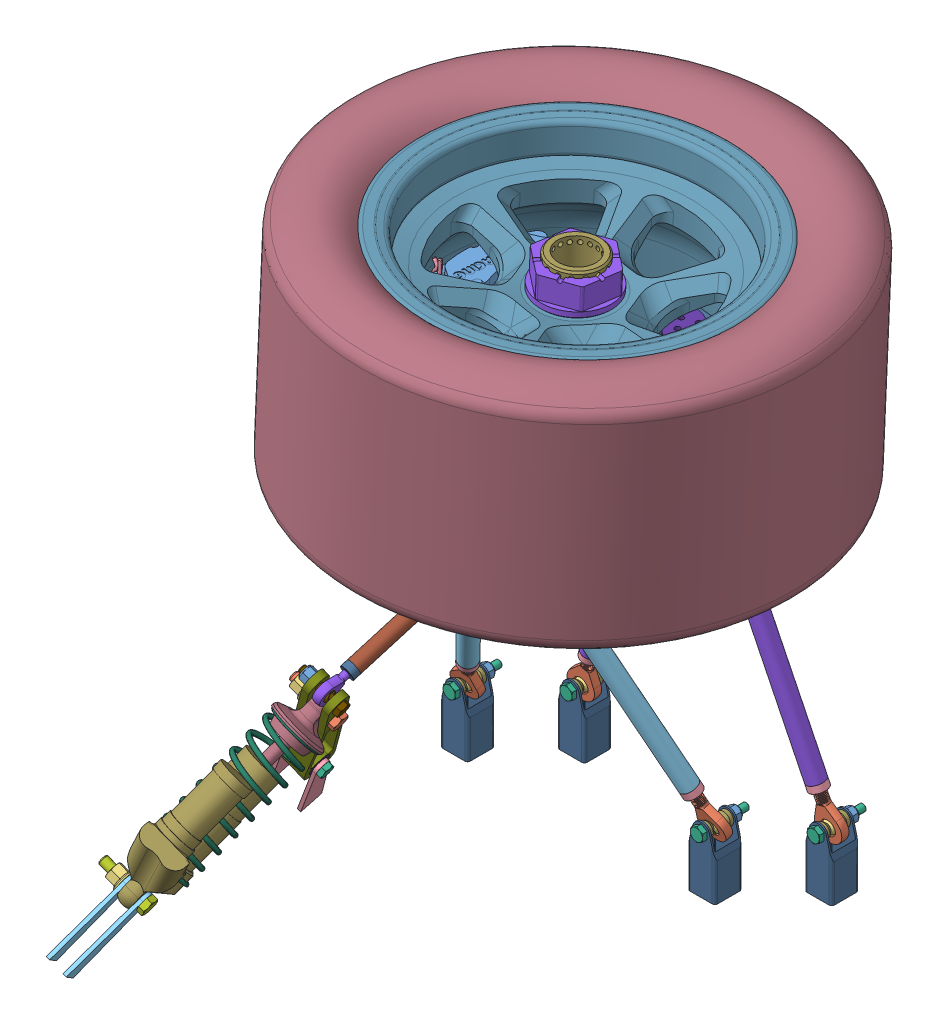
SolidWorks assembly WT-A0100-AC-Unsprung FRONT Axle Asszembly, configuration Default. Lengths in mm.
Overall size (1029.74 758.91 586.73).
149 component instances, 58 part files, 6 mates.
Components (placement in the parent):
- SP-A0200-AA-Front Axle Assembly-1: SP-A0200-AA-Front Axle Assembly [Default] at origin size (928.85 609.3 561.18)
  - Upper A-Arm^SP-A0200-AA-Front Axle Assembly-1: Upper A-Arm^SP-A0200-AA-Front Axle Assembly [Default] at (0 340.1778 -103.3743) x (1 0 0) z (0 -0.807933 0.589274) size (262.57 296.92 200.08) (virtual)
    - SP-Upper Apex Front-1: SP-Upper Apex Front [Default] at (789.6198 444.1063 49.8797) x (0.938572 -0.289882 0.187221) z (0 0.542537 0.840032) size (51.11 64.07 9.53)
    - MirrorFS-MALE ROD END UNF-3A, 0.3125x24-0.25D (XAM-4)1-1: MirrorFS-MALE ROD END UNF-3A, 0.3125x24-0.25D (XAM-4)1 [Default] at (903.9198 182.9597 218.5422) x (-0.938572 -0.289882 0.187221) z (0.345084 -0.78843 0.50921) size (26.22 11.39 62.85)
      - MirrorBody^MirrorFS-MALE ROD END UNF-3A, 0.3125x24-0.25D (XAM-4)1-1: MirrorBody^MirrorFS-MALE ROD END UNF-3A, 0.3125x24-0.25D (XAM-4)1 [Default] at origin size (26.22 9.76 62.85) (virtual)
      - MirrorBall^MirrorFS-MALE ROD END UNF-3A, 0.3125x24-0.25D (XAM-4)1-1: MirrorBall^MirrorFS-MALE ROD END UNF-3A, 0.3125x24-0.25D (XAM-4)1 [Default] x (0.874091 -0.054164 -0.482733) z (-0.485762 -0.097546 -0.868631) size (12.7 9.53 12.7) (virtual)
    - MirrorFS-MALE ROD END UNF-3A, 0.3125x24-0.25D (XAM-4)1-2: MirrorFS-MALE ROD END UNF-3A, 0.3125x24-0.25D (XAM-4)1 [Default] at (675.3198 182.9597 218.5422) x (0.938572 -0.289882 0.187221) z (-0.345084 -0.78843 0.50921) size (26.22 11.39 62.85)
      - MirrorBody^MirrorFS-MALE ROD END UNF-3A, 0.3125x24-0.25D (XAM-4)1-1: MirrorBody^MirrorFS-MALE ROD END UNF-3A, 0.3125x24-0.25D (XAM-4)1 [Default] at origin size (26.22 9.76 62.85) (virtual)
      - MirrorBall^MirrorFS-MALE ROD END UNF-3A, 0.3125x24-0.25D (XAM-4)1-1: MirrorBall^MirrorFS-MALE ROD END UNF-3A, 0.3125x24-0.25D (XAM-4)1 [Default] x (0.874091 -0.054164 -0.482733) z (-0.485762 -0.097546 -0.868631) size (12.7 9.53 12.7) (virtual)
    - SP-10003-AD-Threaded Insert-1: SP-10003-AD-Threaded Insert [A-Arm] at (690.6588 218.0055 195.9078) x (-0.938572 0.289882 -0.187221) z (-0.345084 -0.78843 0.50921) size (15.88 15.88 15.88)
    - SP-10003-AD-Threaded Insert-2: SP-10003-AD-Threaded Insert [A-Arm] at (888.5808 218.0055 195.9078) x (0 0.542537 0.840032) z (0.345084 -0.78843 0.50921) size (15.88 15.88 15.88)
    - SP-Upper A-Arm Tube-1: SP-Upper A-Arm Tube [Default] at (732.4698 313.533 134.2109) x (0 -0.542537 -0.840032) z (0.938572 -0.289882 0.187221) size (15.88 272.31 15.88)
    - SP-Upper A-Arm Tube-2: SP-Upper A-Arm Tube [Default] at (846.7698 313.533 134.2109) x (0 0.542537 0.840032) z (-0.938572 -0.289882 0.187221) size (15.88 272.31 15.88)
    - FS-HIGH MISALIGN SPHERICAL BEARING, 0.375-0.906D (3072-6G)-1: FS-HIGH MISALIGN SPHERICAL BEARING, 0.375-0.906D (3072-6G) [Default] at (789.6198 444.1063 49.8797) x (-0.345084 -0.78843 0.50921) z (-0.938572 0.289882 -0.187221) size (26.46 21.71 26.13)
      - Race^FS-HIGH MISALIGN SPHERICAL BEARING, 0.375-0.906D (3072-6G)-1: Race^FS-HIGH MISALIGN SPHERICAL BEARING, 0.375-0.906D (3072-6G) [Default] at origin size (23.01 8.76 23.01) (virtual)
      - Ball^FS-HIGH MISALIGN SPHERICAL BEARING, 0.375-0.906D (3072-6G)-1: Ball^FS-HIGH MISALIGN SPHERICAL BEARING, 0.375-0.906D (3072-6G) [Default] x (0.359576 -0.008176 0.93308) z (-0.932238 -0.046516 0.358844) size (19.84 20.65 19.84) (virtual)
  - Lower A-Arm^SP-A0200-AA-Front Axle Assembly-1: Lower A-Arm^SP-A0200-AA-Front Axle Assembly [Default] at (0 -0.114 0.1797) x (1 0 0) z (0 0.000904 1) size (261.54 401.37 64.51) (virtual)
    - SP-Front Lower A-Arm Tube-2: SP-Front Lower A-Arm Tube [Default] at (844.893 441.1433 99.9128) x (0.296605 -0.948118 -0.114444) z (0 -0.119836 0.992794) size (339.15 15.88 15.88)
    - MirrorFS-MALE ROD END UNF-3A, 0.3125x24-0.25D (XAM-4)1-1: MirrorFS-MALE ROD END UNF-3A, 0.3125x24-0.25D (XAM-4)1 [Default] at (912.4748 225.1139 73.8367) x (0.955 0.294468 0.035544) z (0.296605 -0.948118 -0.114444) size (26.22 11.39 62.85)
      - MirrorBody^MirrorFS-MALE ROD END UNF-3A, 0.3125x24-0.25D (XAM-4)1-1: MirrorBody^MirrorFS-MALE ROD END UNF-3A, 0.3125x24-0.25D (XAM-4)1 [Default] at origin size (26.22 9.76 62.85) (virtual)
      - MirrorBall^MirrorFS-MALE ROD END UNF-3A, 0.3125x24-0.25D (XAM-4)1-1: MirrorBall^MirrorFS-MALE ROD END UNF-3A, 0.3125x24-0.25D (XAM-4)1 [Default] x (0.874091 -0.054164 -0.482733) z (-0.485762 -0.097546 -0.868631) size (12.7 9.53 12.7) (virtual)
    - MirrorFS-MALE ROD END UNF-3A, 0.3125x24-0.25D (XAM-4)1-2: MirrorFS-MALE ROD END UNF-3A, 0.3125x24-0.25D (XAM-4)1 [Default] at (683.8748 225.1139 73.8367) x (0.955 -0.294468 -0.035544) z (-0.296605 -0.948118 -0.114444) size (26.22 11.39 62.85)
      - MirrorBody^MirrorFS-MALE ROD END UNF-3A, 0.3125x24-0.25D (XAM-4)1-1: MirrorBody^MirrorFS-MALE ROD END UNF-3A, 0.3125x24-0.25D (XAM-4)1 [Default] at origin size (26.22 9.76 62.85) (virtual)
      - MirrorBall^MirrorFS-MALE ROD END UNF-3A, 0.3125x24-0.25D (XAM-4)1-1: MirrorBall^MirrorFS-MALE ROD END UNF-3A, 0.3125x24-0.25D (XAM-4)1 [Default] x (0.874091 -0.054164 -0.482733) z (-0.485762 -0.097546 -0.868631) size (12.7 9.53 12.7) (virtual)
    - SP-Lower Apex Front-1: SP-Lower Apex Front [Default] at (798.1748 590.481 117.9388) x (0.955 -0.294468 -0.035544) z (0 -0.119836 0.992794) size (48.15 64.07 9.53)
    - SP-10003-AD-Threaded Insert-1: SP-10003-AD-Threaded Insert [A-Arm] at (899.2907 267.2577 78.9237) x (0.955 0.294468 0.035544) z (0.296605 -0.948118 -0.114444) size (15.88 15.88 15.88)
    - SP-10003-AD-Threaded Insert-2: SP-10003-AD-Threaded Insert [A-Arm] at (697.0589 267.2577 78.9237) x (0.955 -0.294468 -0.035544) z (-0.296605 -0.948118 -0.114444) size (15.88 15.88 15.88)
    - FS-HIGH MISALIGN SPHERICAL BEARING, 0.375-0.906D (3072-6G)-1: FS-HIGH MISALIGN SPHERICAL BEARING, 0.375-0.906D (3072-6G) [Default] at (798.1748 590.481 117.9388) x (0.296605 0.948118 0.114444) z (-0.955 0.294468 0.035544) size (26.46 21.71 26.13)
      - Race^FS-HIGH MISALIGN SPHERICAL BEARING, 0.375-0.906D (3072-6G)-1: Race^FS-HIGH MISALIGN SPHERICAL BEARING, 0.375-0.906D (3072-6G) [Default] at origin size (23.01 8.76 23.01) (virtual)
      - Ball^FS-HIGH MISALIGN SPHERICAL BEARING, 0.375-0.906D (3072-6G)-1: Ball^FS-HIGH MISALIGN SPHERICAL BEARING, 0.375-0.906D (3072-6G) [Default] x (0.359576 -0.008176 0.93308) z (-0.932238 -0.046516 0.358844) size (19.84 20.65 19.84) (virtual)
    - SP-Front Lower A-Arm Tube-3: SP-Front Lower A-Arm Tube [Default] at (751.4566 441.1433 99.9128) x (-0.296605 -0.948118 -0.114444) z (0 -0.119836 0.992794) size (339.15 15.88 15.88)
  - SP-C30066-AA-A-Arm Tab Box-2: SP-C30066-AA-A-Arm Tab Box [Default] at (903.9198 253.9613 173.2262) x (0 1 0) z (-1 0 0) size (60.32 25.4 25.4)
  - SP-C30066-AA-A-Arm Tab Box-3: SP-C30066-AA-A-Arm Tab Box [Default] at (675.3198 253.9613 173.2262) x (0 1 0) z (-1 0 0) size (60.32 25.4 25.4)
  - SP-C30066-AA-A-Arm Tab Box-4: SP-C30066-AA-A-Arm Tab Box [Default] at (912.4748 207.6041 73.8128) x (0 1 0) z (-1 0 0) size (60.32 25.4 25.4)
  - SP-C30066-AA-A-Arm Tab Box-5: SP-C30066-AA-A-Arm Tab Box [Default] at (683.8748 207.6041 73.8128) x (0 1 0) z (-1 0 0) size (60.32 25.4 25.4)
  - MirrorSP-30063-AB-Pushrod Tab-1: MirrorSP-30063-AB-Pushrod Tab [Default] at (810.0811 539.62 115.4288) x (1 0 0) z (0 0.104591 -0.994515) size (1.59 15.88 23.81)
  - MirrorSP-30063-AB-Pushrod Tab-2: MirrorSP-30063-AB-Pushrod Tab [Default] at (786.2686 539.62 115.4288) x (1 0 0) z (0 0.104591 -0.994515) size (1.59 15.88 23.81)
  - SP-A0105-AC-Ohlin TTX25 MKII, 200mm-2: SP-A0105-AC-Ohlin TTX25 MKII, 200mm [Default] at (696.4401 277.6233 502.0343) x (0.862886 -0.493364 -0.109636) z (-0.277169 -0.64335 0.713637) size (48.39 85.02 197.6)
    - Shock Body^SP-A0105-AC-Ohlin TTX25 MKII, 200mm-1: Shock Body^SP-A0105-AC-Ohlin TTX25 MKII, 200mm [Default] at origin size (40.76 80 131.7) (virtual)
    - Head^SP-A0105-AC-Ohlin TTX25 MKII, 200mm-1: Head^SP-A0105-AC-Ohlin TTX25 MKII, 200mm [Default] at (0 0 -174.6) size (46 46 119) (virtual)
    - Ball^SP-A0105-AC-Ohlin TTX25 MKII, 200mm-1: Ball^SP-A0105-AC-Ohlin TTX25 MKII, 200mm [Default] at (0 0 -174.6) x (-0.011681 0.107343 0.994153) z (0.993776 0.111394 -0.000351) size (15 15 8) (virtual)
    - Ball^SP-A0105-AC-Ohlin TTX25 MKII, 200mm-2: Ball^SP-A0105-AC-Ohlin TTX25 MKII, 200mm [Default] x (0.079523 -0.862756 -0.499328) z (0.965926 -0.057074 0.252448) size (15 15 8) (virtual)
    - SP-#####-AB-Spring-1: SP-#####-AB-Spring [Default] at (0 0 -151.1) size (48.39 49.05 127.97)
  - Front Rocker Assembly-1: Front Rocker Assembly [Default] at (694.2782 309.5507 341.3462) x (0.862886 -0.493364 -0.109636) z (-0.088476 -0.361041 0.928343) size (45.3 150.81 50.27)
    - SP-Front Rocker-1: SP-Front Rocker [Default] at origin size (25.4 150.81 28.57)
    - FS-BALL BEARING, 0.25ID-0.75OD (60355K702)-1: FS-BALL BEARING, 0.25ID-0.75OD (60355K702) [Default] at (9.1281 0 0) x (0 0 1) z (-1 0 0) size (19.05 19.05 7.14)
    - FS-BALL BEARING, 0.25ID-0.75OD (60355K702)-2: FS-BALL BEARING, 0.25ID-0.75OD (60355K702) [Default] at (-9.1281 0 0) x (0 0 1) z (-1 0 0) size (19.05 19.05 7.14)
    - FS-CADMIUM PLATED C3 HX, 0.25x28-1.41-0.469 (AN4-13A)-1: FS-CADMIUM PLATED C3 HX, 0.25x28-1.41-0.469 (AN4-13A) [Default] at (-3.0226 127 0) x (-1 0 0) z (0 1 0) size (40.18 12.9 11.18)
    - FS-NYLOC G8 HX, 0.25x28-0.3125 (90630A145)-1: FS-NYLOC G8 HX, 0.25x28-0.3125 (90630A145) [Default] at (-12.7 127 0) x (0 1 0) z (0 0 1) size (11.11 7.94 12.83)
    - MirrorFS-ZINC YELLOW CHROMATE C10.9 HX, M8x1.25-40-22 (95327A569)-1: MirrorFS-ZINC YELLOW CHROMATE C10.9 HX, M8x1.25-40-22 (95327A569) [Default] at (-4.65 101.6 0) x (-1 0 0) z (0 0 1) size (45.3 15.01 13)
    - FS-NYLOC FLHX C8, M8x1.25-11.1 (92461A400)-1: FS-NYLOC FLHX C8, M8x1.25-11.1 (92461A400) [Default] at (-23.8 101.6 0) x (0 1 0) z (-1 0 0) size (17.9 17.9 11.1)
  - SP-A0200-Front Rocker Tab Box-1: SP-A0200-Front Rocker Tab Box [Front] at (706.6066 302.5017 339.7797) x (0.862886 -0.493364 -0.109636) z (-0.497595 -0.791354 -0.355188) size (3.17 19.05 82.64)
  - SP-A0200-Front Rocker Tab Box-2: SP-A0200-Front Rocker Tab Box [Front] at (681.9497 316.5996 342.9126) x (0.862886 -0.493364 -0.109636) z (-0.497595 -0.791354 -0.355188) size (3.17 19.05 82.64)
  - SP-A0200-Shock Tab-1: SP-A0200-Shock Tab [Default] at (703.1358 273.795 501.1836) x (0.862886 -0.493364 -0.109636) z (-0.277169 -0.64335 0.713637) size (3.17 23.81 77.22)
  - SP-A0200-Shock Tab-2: SP-A0200-Shock Tab [Default] at (689.4375 281.6271 502.9241) x (0.862886 -0.493364 -0.109636) z (-0.277169 -0.64335 0.713637) size (3.17 23.81 77.22)
  - FS-NYLOC G8 HX, 0.25x28-0.3125 (90630A145)-3: FS-NYLOC G8 HX, 0.25x28-0.3125 (90630A145) [Default] at (675.3198 271.4238 160.5262) x (1 0 0) z (0 1 0) size (11.11 7.94 12.83)
  - FS-NYLOC G8 HX, 0.25x28-0.3125 (90630A145)-4: FS-NYLOC G8 HX, 0.25x28-0.3125 (90630A145) [Default] at (683.8748 225.0666 61.1128) x (1 0 0) z (0 1 0) size (11.11 7.94 12.83)
  - FS-CADMIUM PLATED C3 HEX, 0.25x28-1.65-0.469 (AN4-13A)-1: FS-CADMIUM PLATED C3 HEX, 0.25x28-1.65-0.469 (AN4-13A) [Default] at (903.9198 271.4238 167.1556) x (0 0 -1) z (-1 0 0) size (46.28 12.9 11.18)
  - FS-CADMIUM PLATED C3 HEX, 0.25x28-1.65-0.469 (AN4-13A)-2: FS-CADMIUM PLATED C3 HEX, 0.25x28-1.65-0.469 (AN4-13A) [Default] at (675.3198 271.4238 167.1556) x (0 0 -1) z (-1 0 0) size (46.28 12.9 11.18)
  - FS-CADMIUM PLATED C3 HEX, 0.25x28-1.65-0.469 (AN4-13A)-3: FS-CADMIUM PLATED C3 HEX, 0.25x28-1.65-0.469 (AN4-13A) [Default] at (683.8748 225.0666 67.7422) x (0 0 -1) z (1 0 0) size (46.28 12.9 11.18)
  - FS-CADMIUM PLATED C3 HEX, 0.25x28-1.65-0.469 (AN4-13A)-4: FS-CADMIUM PLATED C3 HEX, 0.25x28-1.65-0.469 (AN4-13A) [Default] at (912.4748 225.0666 67.7422) x (0 0 -1) z (1 0 0) size (46.28 12.9 11.18)
  - FS-CADMIUM PLATED C3 HEX, 0.25x28-1.65-0.469 (AN4-13A)-5: FS-CADMIUM PLATED C3 HEX, 0.25x28-1.65-0.469 (AN4-13A) [Default] at (792.898 537.9596 131.2167) x (-1 0 0) z (0 0.104591 -0.994515) size (46.28 12.9 11.18)
  - FS-CADMIUM PLATED C3 HEX, 0.25x28-1.65-0.469 (AN4-13A)-6: FS-CADMIUM PLATED C3 HEX, 0.25x28-1.65-0.469 (AN4-13A) [Default] at (691.7796 310.9792 341.6636) x (-0.862886 0.493364 0.109636) z (0.505399 0.842338 0.187186) size (46.28 12.9 11.18)
  - FS-ZINC YELLOW CHROMATE C10.9 HX, M8x1.25-40-22 (95327A569)-1: FS-ZINC YELLOW CHROMATE C10.9 HX, M8x1.25-40-22 (95327A569) [Default] at (689.5346 281.5716 502.9117) x (-0.862886 0.493364 0.109636) z (0.422618 0.5854 0.691883) size (45.3 15.01 13)
  - FS-NYLOC FLHX C8, M8x1.25-11.1 (92461A400)-1: FS-NYLOC FLHX C8, M8x1.25-11.1 (92461A400) [Default] at (678.4896 287.8867 504.3151) x (-0.277169 -0.64335 0.713637) z (-0.862886 0.493364 0.109636) size (17.9 17.9 11.1)
  - FS-NYLOC G8 HX, 0.25x28-0.3125 (90630A145)-1: FS-NYLOC G8 HX, 0.25x28-0.3125 (90630A145) [Default] at (903.9198 271.4238 160.5262) x (1 0 0) z (0 1 0) size (11.11 7.94 12.83)
  - FS-NYLOC G8 HX, 0.25x28-0.3125 (90630A145)-2: FS-NYLOC G8 HX, 0.25x28-0.3125 (90630A145) [Default] at (912.4748 225.0666 61.1128) x (1 0 0) z (0 1 0) size (11.11 7.94 12.83)
  - FS-NYLOC G8 HX, 0.25x28-0.3125 (90630A145)-5: FS-NYLOC G8 HX, 0.25x28-0.3125 (90630A145) [Default] at (786.2686 537.9596 131.2167) x (0 0.994515 0.104591) z (0 -0.104591 0.994515) size (11.11 7.94 12.83)
  - Push Rod^SP-A0200-AA-Front Axle Assembly-1: Push Rod^SP-A0200-AA-Front Axle Assembly [Default] at (-52.7488 99.3961 3.2852) x (0.997708 -0.055202 -0.03913) z (0.038438 -0.013527 0.999169) size (65.25 156.18 281.61) (virtual)
    - FS-MALE ROD END UNF-3A, 0.25x28-0.25D (AM-4)-1: FS-MALE ROD END UNF-3A, 0.25x28-0.25D (AM-4) [Default] at (776.2227 359.6297 409.7931) x (-0.286827 -0.837139 -0.465756) z (0.150966 0.440611 -0.884913) size (19.32 14.06 49.44)
      - Body^FS-MALE ROD END UNF-3A, 0.25x28-0.25D (AM-4)-2: Body^FS-MALE ROD END UNF-3A, 0.25x28-0.25D (AM-4) [Default] at origin size (19.32 7.2 49.44) (virtual)
      - Ball^FS-MALE ROD END UNF-3A, 0.25x28-0.25D (AM-4)-2: Ball^FS-MALE ROD END UNF-3A, 0.25x28-0.25D (AM-4) [Default] x (0.09633 0.218783 0.971007) z (-0.984027 0.167661 0.059845) size (12.7 9.53 12.7) (virtual)
    - FS-MALE ROD END UNF-3A, 0.25x28-0.25D (AM-4)-2: FS-MALE ROD END UNF-3A, 0.25x28-0.25D (AM-4) [Default] at (819.7582 486.6934 154.6011) x (0.286827 0.837139 0.465756) z (-0.150966 -0.440611 0.884913) size (19.32 14.06 49.44)
      - Body^FS-MALE ROD END UNF-3A, 0.25x28-0.25D (AM-4)-2: Body^FS-MALE ROD END UNF-3A, 0.25x28-0.25D (AM-4) [Default] at origin size (19.32 7.2 49.44) (virtual)
      - Ball^FS-MALE ROD END UNF-3A, 0.25x28-0.25D (AM-4)-2: Ball^FS-MALE ROD END UNF-3A, 0.25x28-0.25D (AM-4) [Default] x (0.09633 0.218783 0.971007) z (-0.984027 0.167661 0.059845) size (12.7 9.53 12.7) (virtual)
    - SP-10003-AC-Threaded Insert-1: SP-10003-AC-Threaded Insert [AM-4 Rod End Thread] at (781.4952 375.018 378.8875) x (0.286827 0.837139 0.465756) z (-0.150966 -0.440611 0.884913) size (12.7 12.7 15.88)
    - SP-10003-AC-Threaded Insert-2: SP-10003-AC-Threaded Insert [AM-4 Rod End Thread] at (814.4858 471.3051 185.5067) x (-0.286827 -0.837139 -0.465756) z (0.150966 0.440611 -0.884913) size (12.7 12.7 15.88)
    - SP-A0200-Front Push Rod Tube-1: SP-A0200-Front Push Rod Tube [Default] at (797.9905 423.1616 282.1971) x (-0.286827 -0.837139 -0.465756) z (0.946012 -0.32413 0) size (12.7 237.58 12.7)
  - FS-ROD END RETAINING WASHER, 0.25-0.245 (NO PN)-1: FS-ROD END RETAINING WASHER, 0.25-0.245 (NO PN) [Default] at (912.4748 225.0666 62.5733) size (12.7 12.7 6.22)
  - FS-ROD END RETAINING WASHER, 0.25-0.245 (NO PN)-2: FS-ROD END RETAINING WASHER, 0.25-0.245 (NO PN) [Default] at (912.4748 225.0666 85.0523) x (-1 0 0) z (0 0 -1) size (12.7 12.7 6.22)
  - FS-ROD END RETAINING WASHER, 0.25-0.245 (NO PN)-3: FS-ROD END RETAINING WASHER, 0.25-0.245 (NO PN) [Default] at (903.9198 271.4238 161.9867) size (12.7 12.7 6.22)
  - FS-ROD END RETAINING WASHER, 0.25-0.245 (NO PN)-4: FS-ROD END RETAINING WASHER, 0.25-0.245 (NO PN) [Default] at (903.9198 271.4238 184.4657) x (-1 0 0) z (0 0 -1) size (12.7 12.7 6.22)
  - FS-ROD END RETAINING WASHER, 0.25-0.245 (NO PN)-5: FS-ROD END RETAINING WASHER, 0.25-0.245 (NO PN) [Default] at (683.8748 225.0666 62.5733) size (12.7 12.7 6.22)
  - FS-ROD END RETAINING WASHER, 0.25-0.245 (NO PN)-6: FS-ROD END RETAINING WASHER, 0.25-0.245 (NO PN) [Default] at (683.8748 225.0666 85.0523) x (-1 0 0) z (0 0 -1) size (12.7 12.7 6.22)
  - FS-ROD END RETAINING WASHER, 0.25-0.245 (NO PN)-7: FS-ROD END RETAINING WASHER, 0.25-0.245 (NO PN) [Default] at (675.3198 271.4238 161.9867) size (12.7 12.7 6.22)
  - FS-ROD END RETAINING WASHER, 0.25-0.245 (NO PN)-8: FS-ROD END RETAINING WASHER, 0.25-0.245 (NO PN) [Default] at (675.3198 271.4238 184.4657) x (-1 0 0) z (0 0 -1) size (12.7 12.7 6.22)
  - FS-ROD END RETAINING WASHER, 0.25-0.245 (NO PN)-9: FS-ROD END RETAINING WASHER, 0.25-0.245 (NO PN) [Default] at (810.2081 537.9596 131.2167) x (0 0.994515 0.104591) z (-1 0 0) size (12.7 12.7 6.22)
  - FS-ROD END RETAINING WASHER, 0.25-0.245 (NO PN)-10: FS-ROD END RETAINING WASHER, 0.25-0.245 (NO PN) [Default] at (787.7291 537.9596 131.2167) x (0 -0.994515 -0.104591) z (1 0 0) size (12.7 12.7 6.22)
- WT-A0100-AG-Corner Assembly-1: WT-A0100-AG-Corner Assembly [Front Left Corner Assembly] at (-13.9216 21.8764 -3.3679) x (0.999396 -0.032062 0.013421) z (-0.013003 0.013211 0.999828) size (999.8 719.84 564.21)
  - WT-00202-AA-Hoosier R25B 16x7_5-10-1: WT-00202-AA-Hoosier R25B 16x7_5-10 [Default] at (794.0641 613.0878 197.9453) x (0 0 -1) z (0 -1 0) size (411.48 411.48 213.5)
  - WT-00201-AA-OZ Centerlock 10in Wheel-1: WT-00201-AA-OZ Centerlock 10in Wheel [Default] at (794.0641 635.0878 197.9453) x (0.604277 0 -0.796774) z (0 1 0) size (288.79 288.79 189.86)
  - WT-10105-AA-Drive Pin-8: WT-10105-AA-Drive Pin [Default] at (833.7508 635.0878 202.9426) x (0.931762 0 -0.363068) z (0.363068 0 0.931762) size (12.67 23.01 11.95)
  - BR-20602-AC-Brake Hat-2: BR-20602-AC-Brake Hat [Default] at (794.0641 608.9576 197.9453) x (-0.604278 0 0.796774) z (-0.796774 0 -0.604278) size (120.29 4.76 113.7)
  - BR-20601-AA-Brake Rotor-1: BR-20601-AA-Brake Rotor [Default] at (794.0641 608.9576 197.9453) x (-0.992165 0 -0.124933) z (0.124933 0 -0.992165) size (190.5 4.76 190.5)
  - CP4227-2S0-1: CP4227-2S0 [Default] at (809.9391 608.9576 197.9254) x (0.998694 0 0.051087) z (-0.051087 0 0.998694) size (71.54 66.42 130.94)
    - CP4227-2S0.STEP-1: CP4227-2S0.STEP [Default] x (0 0 -1) z (0 -1 0) size (130.94 71.54 66.42)
      - CP4227-101.STEP-1: CP4227-101.STEP [Default] at origin size (112 60.5 34.68)
      - CP4227-102.STEP-1: CP4227-102.STEP [Default] x (-1 0 0) z (0 0 -1) size (109 47.57 30.98)
      - cp3049-40a_CP4226-103.STEP-1: cp3049-40a_CP4226-103.STEP [Default] at (-23.4668 -94.12 -10.305) size (25.2 25.2 14.87)
      - cp3049-40a_CP4226-103.STEP-2: cp3049-40a_CP4226-103.STEP [Default] at (-23.4668 -94.12 10.305) x (-0.98369 0.179874 0) z (0 0 -1) size (25.2 25.2 14.87)
      - cp3049-40a_CP4226-103.STEP-3: cp3049-40a_CP4226-103.STEP [Default] at (23.4668 -94.12 10.305) x (-0.960147 0.279495 0) z (0 0 -1) size (25.2 25.2 14.87)
      - cp3049-40a_CP4226-103.STEP-4: cp3049-40a_CP4226-103.STEP [Default] at (23.4668 -94.12 -10.305) size (25.2 25.2 14.87)
      - cp3838-M08x1.25m_CP4477-110.STEP-1: cp3838-M08x1.25m_CP4477-110.STEP [Default] at (-41.1 -109.6 19.55) x (-0.998897 0.046962 0) z (0 0 -1) size (13 13 46)
      - cp3838-M08x1.25m_CP4477-110.STEP-2: cp3838-M08x1.25m_CP4477-110.STEP [Default] at (0 -116.83 19.55) x (-0.99038 0.138378 0) z (0 0 -1) size (13 13 46)
      - cp3838-M08x1.25m_CP4477-110.STEP-3: cp3838-M08x1.25m_CP4477-110.STEP [Default] at (41.1 -109.6 19.55) x (-1 -0.000032 0) z (0 0 -1) size (13 13 46)
      - cp4226-104_CP4226-104.STEP-1: cp4226-104_CP4226-104.STEP [Default] at (-29.0318 -116.44 -31.75) x (0 0 1) z (1 0 0) size (61.35 20.1 3)
      - cp4226-104_CP4226-104.STEP-2: cp4226-104_CP4226-104.STEP [Default] at (29.0318 -116.44 -31.75) x (0 0 1) z (1 0 0) size (61.35 20.1 3)
      - CP4469-101.STEP-1: CP4469-101.STEP [Default] at (-65.47 -82.62 -23.98) x (0 0.474307 -0.88036) z (1 0 0) size (9.24 8.21 29.15)
      - CP4469-101.STEP-2: CP4469-101.STEP [Default] at (65.47 -82.62 -23.98) x (0 0.509894 0.860237) z (-1 0 0) size (9.24 8.21 29.15)
      - CP4226-4m.STEP-1: CP4226-4m.STEP [Default] at (10.0433 -40.2815 10.305) x (0.970296 0.241922 0) z (0 0 -1) size (39.7 43.64 7)
      - CP4226-4m.STEP-2: CP4226-4m.STEP [Default] at (10.0433 -40.2815 -10.305) x (-0.970296 -0.241922 0) z (0 0 1) size (39.7 43.64 7)
      - CP4226-4m.STEP-3: CP4226-4m.STEP [Default] at (-10.0433 -40.2815 -10.305) x (-0.970296 0.241922 0) z (0 0 1) size (39.7 43.64 7)
      - CP4226-4m.STEP-4: CP4226-4m.STEP [Default] at (-10.0433 -40.2815 10.305) x (0.970296 -0.241922 0) z (0 0 -1) size (39.7 43.64 7)
  - WT-20104-AC-Sensor Ring-1: WT-20104-AC-Sensor Ring [Default] at (794.0641 606.5764 197.9453) x (-0.992165 0 -0.124933) z (0 -1 0) size (113.66 114.3 1.59)
  - WT-10105-AA-Drive Pin-18: WT-10105-AA-Drive Pin [Default] at (-39.6866 22.1233 -4.4197) x (-0.931762 -0.009504 0.362944) z (-0.363068 0.024391 -0.931443) size (12.67 23.01 11.95) (suppressed, hidden)
  - WT-10105-AA-Drive Pin-19: WT-10105-AA-Drive Pin [Default] at (4.9973 23.0313 -39.0971) x (-0.363068 0.024391 -0.931443) z (0.931762 0.009504 -0.362944) size (12.67 23.01 11.95) (suppressed, hidden)
  - WT-10105-AA-Drive Pin-20: WT-10105-AA-Drive Pin [Default] at (39.6866 21.8616 5.5715) x (0.931762 0.009504 -0.362944) z (0.363068 -0.024391 0.931443) size (12.67 23.01 11.95) (suppressed, hidden)
  - WT-10102-AA-Centerlock Nut-1: WT-10102-AA-Centerlock Nut [Default] at (794.0641 685.7073 197.9453) x (-0.796774 0 -0.604278) z (0.604278 0 -0.796774) size (66 31.86 66)
  - WT-AA-Camber Block-1: WT-AA-Camber Block [Default] at (789.2314 585.9914 292.4205) x (-0.998694 0 -0.051087) z (-0.048552 -0.311078 0.949143) size (47.63 44.45 33.35)
  - WT-AF-Upright-1: WT-AF-Upright [Default] at (794.0641 576.6365 197.9453) x (-0.998694 0 -0.051087) z (-0.051087 0 0.998694) size (101.76 54.87 213.53)
  - 1985-1932-TheTimkenCompany-3D-01-05-2023.stp-1: 1985-1932-TheTimkenCompany-3D-01-05-2023.stp [Default] at (794.0641 573.7663 197.9453) x (0 -1 0) z (0.770724 0 0.637169) size (21.39 58.74 58.74)
  - WT-10101-AB-Wheel Hub Front-1: WT-10101-AB-Wheel Hub Front [Front] at (794.0641 623.6579 197.9453) x (0.992165 0 0.124933) z (-0.124933 0 0.992165) size (96.32 137.41 96.32)
  - 1985-1932-TheTimkenCompany-3D-01-05-2023.stp-2: 1985-1932-TheTimkenCompany-3D-01-05-2023.stp [Default] at (794.0641 579.5067 197.9453) x (0 1 0) z (0.648222 0 -0.761452) size (21.39 58.74 58.74)
  - WT-10106-AB-Backing Plate-1: WT-10106-AB-Backing Plate [Default] at (794.0641 553.2364 197.9453) x (0.757216 0 -0.653165) z (0.653165 0 0.757216) size (58.23 5.08 58.23)
  - WT-AA- Front Grease Seal-2: WT-AA- Front Grease Seal [Default] at (794.0641 603.8823 197.9453) x (0.615562 0 0.788088) z (0.788088 0 -0.615562) size (58.74 7.71 58.74)
  - WT-A8###-AA-Front Toe Bracket-1: WT-A8###-AA-Front Toe Bracket [Default] at (812.7128 552.1191 140.0203) x (0.998694 0 0.051087) z (-0.051087 0 0.998694) size (38.1 31.83 47.62)
    - WT-FB-Toe Base Plate-1: WT-FB-Toe Base Plate [Default] at (22.5935 33.4208 28.102) size (3.17 31.83 47.62)
    - WT-FB-Toe Bottom Clevis-1: WT-FB-Toe Bottom Clevis [Default] at (55.0491 23.7722 13.7805) size (38.1 31.83 3.17)
    - WT-FB-Toe Top Clevis-1: WT-FB-Toe Top Clevis [Default] at (52.058 13.9287 39.1805) size (38.1 31.83 3.17)
  - BR-20603-AA-Floating Bobbins-1: BR-20603-AA-Floating Bobbins [Default] at (853.9165 609.1322 205.4819) x (1 0 0.000002) z (-0.000002 0 1) size (12.7 8.29 12.7)
  - 97447A110_Aluminum Blind Rivets with Aluminum Mandrel-1: 97447A110_Aluminum Blind Rivets with Aluminum Mandrel [97447A110] at (835.6457 604.9889 203.1813) x (0.907339 0 0.4204) z (0 -1 0) size (5.03 5.03 11.56)
  - 97447A110_Aluminum Blind Rivets with Aluminum Mandrel-2: 97447A110_Aluminum Blind Rivets with Aluminum Mandrel [97447A110] at (819.3894 604.9889 164.5525) x (0.817747 0 -0.575578) z (0 -1 0) size (5.03 5.03 11.56)
  - 97447A110_Aluminum Blind Rivets with Aluminum Mandrel-3: 97447A110_Aluminum Blind Rivets with Aluminum Mandrel [97447A110] at (777.8077 604.9889 159.3166) x (-0.089592 0 -0.995979) z (0 -1 0) size (5.03 5.03 11.56)
  - 97447A110_Aluminum Blind Rivets with Aluminum Mandrel-4: 97447A110_Aluminum Blind Rivets with Aluminum Mandrel [97447A110] at (752.4825 604.9889 192.7094) x (-0.907339 0 -0.4204) z (0 -1 0) size (5.03 5.03 11.56)
  - 97447A110_Aluminum Blind Rivets with Aluminum Mandrel-5: 97447A110_Aluminum Blind Rivets with Aluminum Mandrel [97447A110] at (768.7388 604.9889 231.3381) x (-0.817747 0 0.575578) z (0 -1 0) size (5.03 5.03 11.56)
  - 97447A110_Aluminum Blind Rivets with Aluminum Mandrel-6: 97447A110_Aluminum Blind Rivets with Aluminum Mandrel [97447A110] at (810.3204 604.9889 236.574) x (0.089592 0 0.995979) z (0 -1 0) size (5.03 5.03 11.56)
  - BR-20603-AA-Floating Bobbins-2: BR-20603-AA-Floating Bobbins [Default] at (817.4634 609.1322 253.5473) x (0.499998 0 0.866027) z (-0.866027 0 0.499998) size (12.7 8.29 12.7)
  - BR-20603-AA-Floating Bobbins-3: BR-20603-AA-Floating Bobbins [Default] at (757.611 609.1322 246.0107) x (-0.500002 0 0.866024) z (-0.866024 0 -0.500002) size (12.7 8.29 12.7)
  - BR-20603-AA-Floating Bobbins-4: BR-20603-AA-Floating Bobbins [Default] at (734.2117 609.1323 190.4087) x (-1 0 -0.000002) z (0.000002 0 -1) size (12.7 8.29 12.7)
  - BR-20603-AA-Floating Bobbins-5: BR-20603-AA-Floating Bobbins [Default] at (770.6648 609.1323 142.3433) x (-0.499998 0 -0.866027) z (0.866027 0 -0.499998) size (12.7 8.29 12.7)
  - BR-20603-AA-Floating Bobbins-6: BR-20603-AA-Floating Bobbins [Default] at (830.5172 609.1323 149.8799) x (0.500002 0 -0.866024) z (0.866024 0 0.500002) size (12.7 8.29 12.7)
  - WT-10105-AA-Drive Pin-21: WT-10105-AA-Drive Pin [Default] at (789.0668 635.0878 237.632) x (0.363068 0 0.931762) z (-0.931762 0 0.363068) size (12.67 23.01 11.95)
  - WT-10105-AA-Drive Pin-22: WT-10105-AA-Drive Pin [Default] at (754.3774 635.0878 192.948) x (-0.931762 0 0.363068) z (-0.363068 0 -0.931762) size (12.67 23.01 11.95)
  - WT-10105-AA-Drive Pin-23: WT-10105-AA-Drive Pin [Default] at (799.0614 635.0879 158.2587) x (-0.363068 0 -0.931762) z (0.931762 0 -0.363068) size (12.67 23.01 11.95)
  - 93070A181_Alloy Steel Low-Profile Socket Head Screw-1: 93070A181_Alloy Steel Low-Profile Socket Head Screw [93070A181] at (740.9846 582.6176 146.3354) x (0 -1 0) z (0 0 1) size (45.29 13 13)
  - 93070A181_Alloy Steel Low-Profile Socket Head Screw-2: 93070A181_Alloy Steel Low-Profile Socket Head Screw [93070A181] at (736.0803 582.6176 242.2101) x (0 -1 0) z (0 0 1) size (45.29 13 13)
  - FS-Jet Nut, M8x1.25 (MJET-M8X1.25)-1: FS-Jet Nut, M8x1.25 (MJET-M8X1.25) [Default] at (736.0803 582.4576 242.2101) x (0.837169 0 0.546944) z (0 -1 0) size (13.6 13.6 7)
  - FS-Jet Nut, M8x1.25 (MJET-M8X1.25)-2: FS-Jet Nut, M8x1.25 (MJET-M8X1.25) [Default] at (740.9846 582.4576 146.3354) x (-0.837169 0 -0.546944) z (0 -1 0) size (13.6 13.6 7)
  - 91251A350_Black-Oxide Alloy Steel Socket Head Screw-1: 91251A350_Black-Oxide Alloy Steel Socket Head Screw [91251A350] at (832.8998 569.9824 188.2666) x (0.051087 0 -0.998694) z (0.998694 0 0.051087) size (7.94 7.94 16.01)
Mates (geometry in assembly coordinates):
- Coincident1: coincident aligned: plane of SP-A0200-AA-Front Axle Assembly-1 through (0 0 0) normal (0 0 1)
- Coincident2: coincident aligned: plane of SP-A0200-AA-Front Axle Assembly-1 through (0 0 0) normal (0 1 0)
- Coincident3: coincident aligned: plane of SP-A0200-AA-Front Axle Assembly-1 through (0 0 0) normal (1 0 0)
- Coincident4: coincident: point of SP-A0200-AA-Front Axle Assembly-1; point of WT-A0100-AG-Corner Assembly-1
- Coincident6: coincident: point of SP-A0200-AA-Front Axle Assembly-1; point of WT-A0100-AG-Corner Assembly-1
- Coincident10: coincident: point of SP-A0200-AA-Front Axle Assembly-1; point of WT-A0100-AG-Corner Assembly-1
